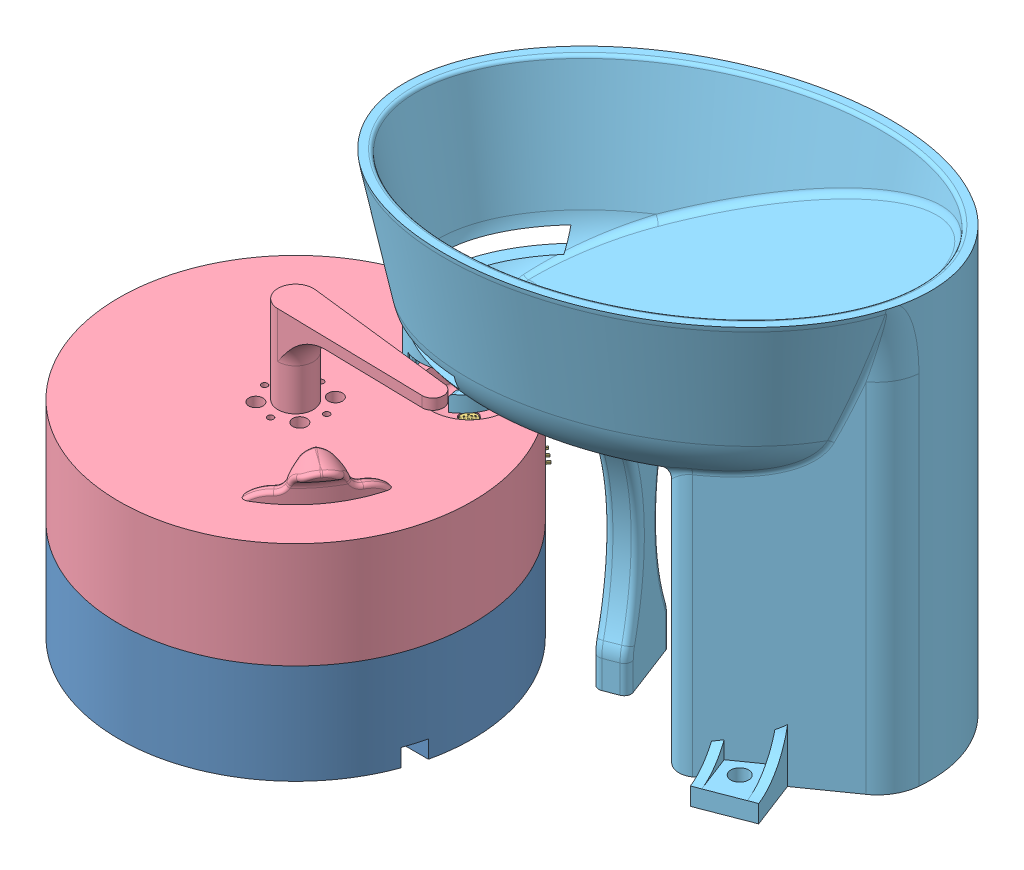
SolidWorks assembly dispenser asm, configuration Default. Lengths in mm.
Overall size (213.97 124.73 185.02).
5 component instances, 5 part files, 10 mates.
Components (placement in the parent):
- Motor fixed flat-1: Motor fixed flat [Default] at origin size (100 28.3 100)
- XL-430-1: XL-430 [기본] at (0 27 0) x (1 0 0) z (0 1 0) size (28.5 46.5 37.91)
- CDS module-1: CDS module [기본] at (22.4408 40.9824 -27.3794) x (-0.628428 0 0.777868) z (-0.777868 0 -0.628428) size (25.25 16.96 14.5)
- Rotating plate-1: Rotating plate [Default] at (0 34 0) x (0.777868 0 0.628428) z (-0.628428 0 0.777868) size (100 54.77 100)
- stone case-1: stone case [Default] at (62.206 125.7 -43.1881) x (0.933336 0 -0.359003) z (0.359003 0 0.933336) size (138.78 124.73 102)
Mates (geometry in assembly coordinates):
- 평행1: parallel anti-aligned: plane of Motor fixed flat-1 through (15 10 0) normal (-1 0 0); plane of XL-430-1 through (14.25 44 33.25) normal (1 0 0)
- 평행2: parallel anti-aligned: plane of Motor fixed flat-1 through (0 10 -12) normal (0 0 1); plane of XL-430-1 through (12.25 44 -11.25) normal (0 0 -1)
- 동심1: concentric aligned: cylinder of Motor fixed flat-1 through (0 -1.3 0) axis (0 1 0) radius 50; cylinder of XL-430-1 through (0 42.5 0) axis (0 1 0) radius 10.25
- 일치3: coincident anti-aligned: plane of Motor fixed flat-1 through (0 10 0) normal (0 1 0); plane of XL-430-1 through (0 10 0) normal (0 -1 0)
- 평행3: parallel anti-aligned: plane of CDS module-1 through (24.3712 48.1812 -27.9669) normal (0.628428 0 -0.777868); plane of Rotating plate-1 through (23.4216 34 -28.9912) normal (-0.628428 0 0.777868)
- 일치5: coincident anti-aligned: plane of CDS module-1 through (21.9924 56.5652 -25.3315) normal (0 1 0); circle of Rotating plate-1
- 동심2: concentric anti-aligned: cylinder of CDS module-1 through (21.995 56.3874 -27.2254) axis (0 -1 0) radius 2.4892; cylinder of Rotating plate-1 through (21.995 34 -27.2254) axis (0 1 0) radius 2.6892
- 동심3: concentric anti-aligned: cylinder of Motor fixed flat-1 through (0 -1.3 0) axis (0 1 0) radius 50; cylinder of Rotating plate-1 through (0 64 0) axis (0 -1 0) radius 50
- 일치6: coincident anti-aligned: plane of Motor fixed flat-1 through (0 34 0) normal (0 1 0); plane of Rotating plate-1 through (0 34 0) normal (0 -1 0)
- 일치7: coincident aligned: plane of Motor fixed flat-1 through (0 5.7 0) normal (0 -1 0); plane of stone case-1 through (62.206 5.7 -43.1881) normal (0 -1 0)
